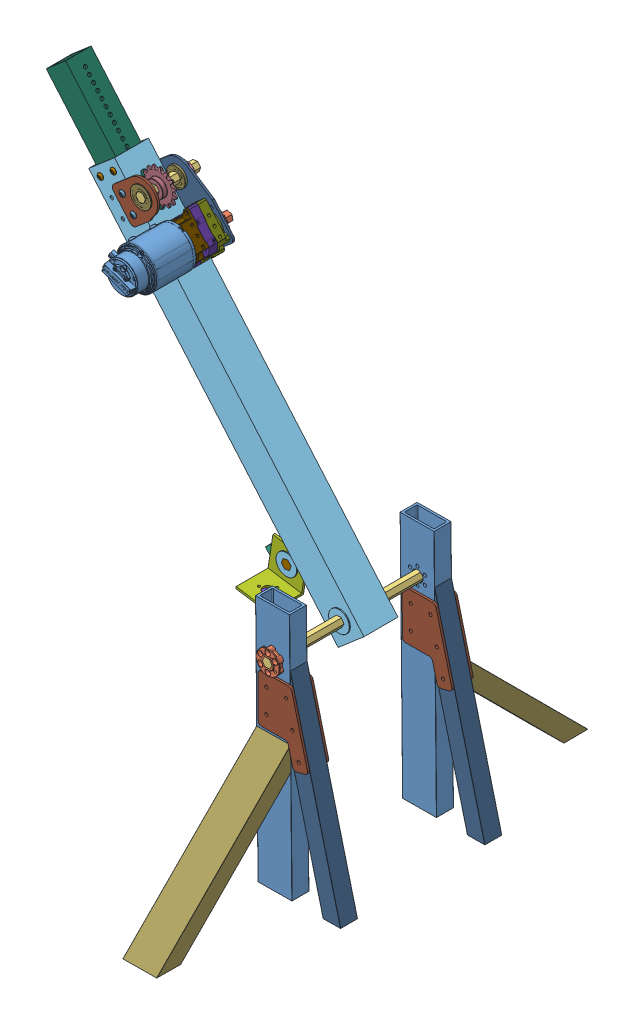
SolidWorks assembly Superstructure, configuration Default. Lengths in mm.
Overall size (550.79 868.94 643.74).
80 component instances, 33 part files, 95 mates.
Components (placement in the parent):
- 3ft 9in Structure Tubing-1: 3ft 9in Structure Tubing [Default] at (63.7822 4129.4809 3.1437) x (0 0 1) z (0.010015 -0.99995 0) size (25.4 50.8 368.3)
- 3ft 9in Structure Tubing-2: 3ft 9in Structure Tubing [Default] at (63.7822 4129.4809 -212.7563) x (0 0 1) z (0.010015 -0.99995 0) size (25.4 50.8 368.3)
- REV Max Hub-3: REV Max Hub [Default] at (39.083 4059.38 -210.5338) x (-0.99995 -0.010015 0) z (0 0 -1) size (34.91 34.92 8.73)
- REV Max Hub-4: REV Max Hub [Default] at (39.083 4059.38 28.5437) x (0.491302 0.870989 0) z (0 0 1) size (34.91 34.92 8.73)
- Dead Axle-1: Dead Axle [Default] at (39.083 4059.38 -219.265) x (0 0 1) z (-0.943614 -0.331047 0) size (256.54 14.38 13.89)
- GOOD Telescoping+Powered+Arm+ASM-3: GOOD Telescoping+Powered+Arm+ASM [Default] at (-316.9253 4473.4855 -96.9323) x (0 0 1) z (-0.65191 0.758296 0) size (167.89 106.2 685.8)
  - Telescoping+Powered+Arm+ASM.stp-1: Telescoping+Powered+Arm+ASM.stp [Default] at origin size (82.02 101.6 1168.4)
    - 2x2tube ASM.stp-1: 2x2tube ASM.stp [Default] at origin size (55.93 50.8 914.4)
      - Slider_Blocks.stp-1: Slider_Blocks.stp [Default] at origin size (17.4 47.5 12.7)
        - Slider_Blocks_4.stp-1: Slider_Blocks_4.stp [Default] at (-0.0635 1254.125 -781.05) x (0 1 0) z (-1 0 0) size (47.5 12.7 17.4)
      - Slider_Blocks_1.stp-1: Slider_Blocks_1.stp [Default] at origin size (17.4 47.5 12.7)
        - Slider_Blocks_4.stp-1: Slider_Blocks_4.stp [Default] at (-0.0635 1254.125 -908.05) x (0 1 0) z (-1 0 0) size (47.5 12.7 17.4)
      - Slider_Blocks_2.stp-1: Slider_Blocks_2.stp [Default] at origin size (17.4 47.5 12.7)
        - Slider_Blocks_4.stp-1: Slider_Blocks_4.stp [Default] at (0.0635 -1254.125 -781.05) x (0 -1 0) z (1 0 0) size (47.5 12.7 17.4)
      - Slider_Blocks_3.stp-1: Slider_Blocks_3.stp [Default] at origin size (17.4 47.5 12.7)
        - Slider_Blocks_4.stp-1: Slider_Blocks_4.stp [Default] at (0.0635 -1254.125 -908.05) x (0 -1 0) z (1 0 0) size (47.5 12.7 17.4)
      - 2x2 long Stick.stp-1: 2x2 long Stick.stp [Default] at origin size (50.8 50.8 914.4)
      - 95185A190_Zinc-Plated Steel Press-Fit Nut for Sheet Metal.stp-1: 95185A190_Zinc-Plated Steel Press-Fit Nut for Sheet Metal.stp [Default] at (-21.5265 12.7 -38.1) x (0 0 -1) z (1 0 0) size (8.64 8.64 3.71)
      - 95185A190_Zinc-Plated Steel Press-Fit Nut for Sheet Metal.stp-2: 95185A190_Zinc-Plated Steel Press-Fit Nut for Sheet Metal.stp [Default] at (-21.5265 12.7 -63.5) x (0 0 -1) z (1 0 0) size (8.64 8.64 3.71)
      - 95185A190_Zinc-Plated Steel Press-Fit Nut for Sheet Metal.stp-3: 95185A190_Zinc-Plated Steel Press-Fit Nut for Sheet Metal.stp [Default] at (-21.5265 12.7 -88.9) x (0 0 -1) z (1 0 0) size (8.64 8.64 3.71)
      - 95185A190_Zinc-Plated Steel Press-Fit Nut for Sheet Metal.stp-4: 95185A190_Zinc-Plated Steel Press-Fit Nut for Sheet Metal.stp [Default] at (-21.5265 12.7 -114.3) x (0 0 -1) z (1 0 0) size (8.64 8.64 3.71)
      - 95185A190_Zinc-Plated Steel Press-Fit Nut for Sheet Metal(Mirror).stp-1: 95185A190_Zinc-Plated Steel Press-Fit Nut for Sheet Metal(Mirror).stp [Default] at (21.5265 12.7 -38.1) x (0 0 -1) z (1 0 0) size (8.64 8.64 3.71)
      - 95185A190_Zinc-Plated Steel Press-Fit Nut for Sheet Metal(Mirror).stp-2: 95185A190_Zinc-Plated Steel Press-Fit Nut for Sheet Metal(Mirror).stp [Default] at (21.5265 12.7 -63.5) x (0 0 -1) z (1 0 0) size (8.64 8.64 3.71)
      - 95185A190_Zinc-Plated Steel Press-Fit Nut for Sheet Metal(Mirror).stp-3: 95185A190_Zinc-Plated Steel Press-Fit Nut for Sheet Metal(Mirror).stp [Default] at (21.5265 12.7 -88.9) x (0 0 -1) z (1 0 0) size (8.64 8.64 3.71)
      - 95185A190_Zinc-Plated Steel Press-Fit Nut for Sheet Metal(Mirror).stp-4: 95185A190_Zinc-Plated Steel Press-Fit Nut for Sheet Metal(Mirror).stp [Default] at (21.5265 12.7 -114.3) x (0 0 -1) z (1 0 0) size (8.64 8.64 3.71)
      - 91255A025_Button Head Hex Drive Screw.stp-1: 91255A025_Button Head Hex Drive Screw.stp [Default] at (-24.3014 -12.7 -12.7) x (0 0 1) z (-1 0 0) size (9.16 9.16 7.33)
      - 91255A025_Button Head Hex Drive Screw.stp-2: 91255A025_Button Head Hex Drive Screw.stp [Default] at (-24.3014 12.7 -12.7) x (0 0 1) z (-1 0 0) size (9.16 9.16 7.33)
      - 91255A025_Button Head Hex Drive Screw.stp-3: 91255A025_Button Head Hex Drive Screw.stp [Default] at (-24.3014 12.7 -139.7) x (0 0 1) z (-1 0 0) size (9.16 9.16 7.33)
      - 91255A025_Button Head Hex Drive Screw.stp-4: 91255A025_Button Head Hex Drive Screw.stp [Default] at (-24.3014 -12.7 -139.7) x (0 0 1) z (-1 0 0) size (9.16 9.16 7.33)
      - 91255A025_Button Head Hex Drive Screw(Mirror).stp-1: 91255A025_Button Head Hex Drive Screw(Mirror).stp [Default] at (24.3014 -12.7 -12.7) x (0 0 1) z (-1 0 0) size (9.16 9.16 7.33)
      - 91255A025_Button Head Hex Drive Screw(Mirror).stp-2: 91255A025_Button Head Hex Drive Screw(Mirror).stp [Default] at (24.3014 12.7 -12.7) x (0 0 1) z (-1 0 0) size (9.16 9.16 7.33)
      - 91255A025_Button Head Hex Drive Screw(Mirror).stp-3: 91255A025_Button Head Hex Drive Screw(Mirror).stp [Default] at (24.3014 12.7 -139.7) x (0 0 1) z (-1 0 0) size (9.16 9.16 7.33)
      - 91255A025_Button Head Hex Drive Screw(Mirror).stp-4: 91255A025_Button Head Hex Drive Screw(Mirror).stp [Default] at (24.3014 -12.7 -139.7) x (0 0 1) z (-1 0 0) size (9.16 9.16 7.33)
    - gear box.stp-1: gear box.stp [Default] at (-25.4 12.7 -38.1) x (0 -1 0) z (1 0 0) size (76.2 113.36 82.02)
      - Selft_drive_Guesset.stp-1: Selft_drive_Guesset.stp [Default] at (12.7 -38.1 25.4) x (0 0 1) z (0 -1 0) size (3.18 76.2 111.91)
        - Selft_drive_Guesset_1.stp-1: Selft_drive_Guesset_1.stp [Default] at (0 -1254.125 -508) x (0 -1 0) z (1 0 0) size (76.2 111.91 3.18)
      - Selfie_drive_guesset_small.stp-1: Selfie_drive_guesset_small.stp [Default] at (12.7 -38.1 25.4) x (0 0 1) z (0 -1 0) size (3.18 64.58 50.8)
        - Selfie_drive_guesset_small_1.stp-1: Selfie_drive_guesset_small_1.stp [Default] at (50.8 -1254.125 -508) x (0 -1 0) z (1 0 0) size (64.58 50.8 3.17)
      - Ball Bearing.stp-1: Ball Bearing.stp [Default] at (-28.067 11.1125 -0.7937) x (1 0 0) z (0 0 -1) size (31.12 31.12 7.94)
      - Ball Bearing.stp-2: Ball Bearing.stp [Default] at (-28.067 11.1125 51.5938) size (31.12 31.12 7.94)
      - hex shaft.stp-1: hex shaft.stp [Default] at (-28.067 11.1125 -388.9375) size (13.74 12.75 73.03) (hidden)
      - 93286A013_Aluminum Washer.stp-1: 93286A013_Aluminum Washer.stp [Default] at (-28.067 11.1125 -5.334) x (0 0 1) z (-1 0 0) size (1.14 17.48 17.48) (hidden)
      - 93286A013_Aluminum Washer.stp-2: 93286A013_Aluminum Washer.stp [Default] at (-28.067 11.1125 68.834) x (0 0 -1) z (1 0 0) size (1.14 17.48 17.48) (hidden)
      - 91255A535_Button Head Hex Drive Screw.stp-1: 91255A535_Button Head Hex Drive Screw.stp [Default] at (-28.067 11.1125 -2.8194) x (1 0 0) z (0 0 -1) size (11.09 11.09 12.88) (hidden)
      - 91255A535_Button Head Hex Drive Screw.stp-2: 91255A535_Button Head Hex Drive Screw.stp [Default] at (-28.067 11.1125 66.3194) size (11.09 11.09 12.88) (hidden)
      - 15 Tooth Sprocket.stp-1: 15 Tooth Sprocket.stp [Default] at (-28.067 11.1125 26.397) size (50.31 50.58 10.68)
      - 91255A262_Button Head Hex Drive Screw.stp-1: 91255A262_Button Head Hex Drive Screw.stp [Default] at (0 76.2 -0.489) x (1 0 0) z (0 0 -1) size (9.16 9.16 10.5)
      - 91255A262_Button Head Hex Drive Screw.stp-2: 91255A262_Button Head Hex Drive Screw.stp [Default] at (0 50.8 -0.489) x (1 0 0) z (0 0 -1) size (9.16 9.16 10.5)
      - 91255A262_Button Head Hex Drive Screw.stp-3: 91255A262_Button Head Hex Drive Screw.stp [Default] at (0 25.4 51.2889) size (9.16 9.16 10.5)
      - 91255A262_Button Head Hex Drive Screw.stp-4: 91255A262_Button Head Hex Drive Screw.stp [Default] at (0 0 -0.489) x (1 0 0) z (0 0 -1) size (9.16 9.16 10.5)
      - 91255A262_Button Head Hex Drive Screw.stp-5: 91255A262_Button Head Hex Drive Screw.stp [Default] at (0 25.4 -0.489) x (1 0 0) z (0 0 -1) size (9.16 9.16 10.5)
      - 91255A262_Button Head Hex Drive Screw.stp-6: 91255A262_Button Head Hex Drive Screw.stp [Default] at (0 0 51.2889) size (9.16 9.16 10.5)
    - 1.5 slide tube.stp-1: 1.5 slide tube.stp [Default] at (-19.05 -19.05 -914.4) size (38.1 38.1 1168.4)
  - gearbox 1-1: gearbox 1 [Default] at (-15.875 50.8 -111.9149) x (-1 0 0) z (0 0 -1) size (23.2 50.8 61.92)
  - gearbox 2-2: gearbox 2 [Default] at (0 50.8 -111.9149) x (0 0 1) z (-1 0 0) size (61.91 50.8 16.85)
  - gearbox 3-1: gearbox 3 [Default] at (15.875 50.8 -111.9149) x (0 0 1) z (-1 0 0) size (61.91 50.8 19.05)
  - Falcon 500, Powered by Talon FX (Rev 3) (217-6515).step-1: Falcon 500, Powered by Talon FX (Rev 3) (217-6515).step [Default] at (86.15 50.8 -111.9149) x (0 0 1) z (-1 0 0) size (62.05 60 125.3)
  - 1in hex axle-1: 1in hex axle [Default] at (-52.3875 50.8003 -111.9276) x (0 -0.481071 -0.876682) z (1 0 0) size (14.66 12.7 38.1)
  - 3.25in hex axle-1: 3.25in hex axle [Default] at (-52.3875 40.7543 -49.2345) x (0 -0.866025 0.5) z (1 0 0) size (14.66 12.7 82.55)
  - 18 tooth sprocket.step-1: 18 tooth sprocket.step [Default] at (-34.29 50.8025 -112.0292) x (0 -0.481071 -0.876682) z (1 0 0) size (39.38 39.82 10.29)
  - 18 tooth sprocket.step-2: 18 tooth sprocket.step [Default] at (-31.5595 40.8051 -49.1465) x (0 0 1) z (-1 0 0) size (39.38 39.82 10.29)
  - Hex Bearing-1: Hex Bearing [Default] at (-18.9967 0 -546.1) x (0 0.175573 0.984466) z (-1 0 0) size (31.12 31.12 7.93)
  - Hex Bearing-2: Hex Bearing [Default] at (18.9967 0 -546.1) x (0 0.878416 0.477897) z (1 0 0) size (31.12 31.12 7.93)
- Arm Mounting Place-3: Arm Mounting Place [Default] at (-51.8162 4048.2259 -109.6323) x (0 0 1) z (-0.65191 0.758296 0) size (127 87.71 84.27)
  - 2x2x2 with holes-1: 2x2x2 with holes [Default] at origin size (25.4 50.8 50.8)
  - Hinge L Bracket-1: Hinge L Bracket [Default] at (-50.8 21.4015 -11.4442) x (1 0 0) z (0 -0.650005 0.75993) size (50.8 50.8 50.8)
  - Hinge L Bracket-2: Hinge L Bracket [Default] at (76.2 -11.6187 27.1602) x (-1 0 0) z (0 0.650005 -0.75993) size (50.8 50.8 50.8)
  - Hex Bearing-1: Hex Bearing [Default] at (3.2283 25.4 25.4) x (0 0 1) z (-1 0 0) size (31.12 31.12 7.93)
  - Hex Bearing-2: Hex Bearing [Default] at (22.1717 25.4 25.4) x (0 0 -1) z (1 0 0) size (31.12 31.12 7.93)
  - 6350K151_3 8 -12 Thread Flange Nut for Fast-Travel Ultra-Precision Lead Screw-1: 6350K151_3 8 -12 Thread Flange Nut for Fast-Travel Ultra-Precision Lead Screw [6350K151] at (-27.9908 4.8914 7.858) x (0 -0.75993 -0.650005) z (-0.733019 0.442138 -0.51691) size (26.34 28.18 28.18)
  - 6350K151_3 8 -12 Thread Flange Nut for Fast-Travel Ultra-Precision Lead Screw-2: 6350K151_3 8 -12 Thread Flange Nut for Fast-Travel Ultra-Precision Lead Screw [6350K151] at (53.3908 4.8914 7.858) x (0 -0.75993 -0.650005) z (0.222567 0.633701 -0.740869) size (26.34 28.18 28.18)
  - 2.5in Axle-1: 2.5in Axle [Default] at (30.099 25.4 25.4) x (0 0.979457 0.201651) z (0 -0.201651 0.979457) size (13.92 34.29 14.36)
- Back Support-1: Back Support [Default] at (-97.4015 4590.0884 -187.3563) x (0 0 -1) z (0.246763 -0.969076 0) size (25.4 25.4 304.68)
- Back Support-2: Back Support [Default] at (-97.0045 4590.0924 28.5437) x (0 0 -1) z (0.246763 -0.969076 0) size (25.4 25.4 304.68)
- Back Support Bracket-1: Back Support Bracket [Default] at (22.9442 3912.6818 28.5437) x (0.999975 0.007087 0) z (0 0 1) size (73.62 105.21 3.17)
- Back Support Bracket-2: Back Support Bracket [Default] at (22.9442 3912.6818 -0.0313) x (0.999975 0.007087 0) z (0 0 1) size (73.62 105.21 3.17)
- Back Support Bracket-3: Back Support Bracket [Default] at (22.5704 3912.5866 -187.3563) x (0.999975 0.007087 0) z (0 0 1) size (73.62 105.21 3.17)
- Back Support Bracket-4: Back Support Bracket [Default] at (22.5704 3912.5866 -215.9313) x (0.999975 0.007087 0) z (0 0 1) size (73.62 105.21 3.17)
- Angled 18in 2x1-1: Angled 18in 2x1 [Default] at (16.6605 3761.9454 -413.3497) x (0.007081 -0.707071 0.707107) z (-0.007081 0.707071 0.707107) size (25.4 50.8 283.68)
- Angled 18in 2x1-2: Angled 18in 2x1 [Default] at (14.6641 3961.2865 28.5437) x (0.007125 -0.711481 -0.70267) z (0.007037 -0.702634 0.711516) size (25.4 50.8 283.68)
Mates (geometry in assembly coordinates):
- Coincident11: coincident: plane of 3ft 9in Structure Tubing-1 through (82.0968 2300.7726 3.3977) normal (0.99995 0.010015 0); plane of 3ft 9in Structure Tubing-2 through (82.0968 2300.7726 -212.5023) normal (0.99995 0.010015 0)
- Coincident15: coincident anti-aligned: plane of 3ft 9in Structure Tubing-1 through (63.5282 4129.4784 3.3977) normal (-0.010015 0.99995 0); plane of Top Connector-1 through (80.3407 4110.2202 1616.0437) normal (0.010015 -0.99995 0)
- Coincident16: coincident aligned: plane of 3ft 9in Structure Tubing-1 through (31.2993 2300.2639 3.3977) normal (-0.99995 -0.010015 0); plane of Top Connector-1 through (29.5433 4109.7115 1616.0437) normal (-0.99995 -0.010015 0)
- Coincident13: coincident aligned: plane of 3ft 9in Structure Tubing-2 through (81.8428 2300.7701 -212.7563) normal (0 0 -1); plane of Back Support-1 through (354.1246 2817.9051 -212.7563) normal (0 0 -1)
- Coincident17: coincident anti-aligned: plane of Back Support-1 through (354.1246 2817.9051 -187.3563) normal (0 0 1); plane of Back Support Connector-1 through (222.6392 3263.2808 -187.3563) normal (0 0 -1)
- Coincident18: coincident aligned: plane of Back Support-1 through (378.493 2824.1102 -187.6103) normal (0.969076 0.246763 0); plane of Back Support Connector-1 through (246.9894 3269.557 1641.4437) normal (0.968351 0.249592 0)
- Distance3: distance = 228.6 mm: line of Back Support Connector-1 through (246.9894 3269.557 3.6517) axis (0 0 -1); line of Back Support-2 through (140.0879 3761.9266 28.2897) axis (0 0 -1)
- Coincident21: coincident anti-aligned: plane of Back Support-2 through (354.5216 2817.909 3.1437) normal (0 0 -1); plane of Back Support Connector-2 through (137.2722 3593.4645 3.1437) normal (0 0 1)
- Coincident22: coincident aligned: plane of Back Support-2 through (378.89 2824.1141 28.2897) normal (0.969076 0.246763 0); plane of Back Support Connector-2 through (161.805 3600.0501 1640.9357) normal (0.968351 0.249592 0)
- Distance4: distance = 228.6 mm: line of Back Support Connector-2 through (155.5921 3624.1543 3.1437) axis (0 0 -1); line of Back Support-2 through (64.9033 4057.1885 28.2897) axis (0 0 -1)
- Coincident29: coincident anti-aligned: plane of 3ft 9in Structure Tubing-2 through (81.8428 2300.7701 -212.7563) normal (0 0 -1); plane of REV Max Hub-1 through (63.7027 4115.5685 -236.4913) normal (0 0 1)
- Coincident32: coincident anti-aligned: plane of 3ft 9in Structure Tubing-1 through (81.8428 2300.7701 28.5437) normal (0 0 1); plane of REV Max Hub-2 through (63.7027 4115.5685 4.8087) normal (0 0 -1)
- Concentric5: concentric anti-aligned: circle of 3ft 9in Structure Tubing-1; circle of REV Max Hub-2
- Concentric6: concentric anti-aligned: circle of 3ft 9in Structure Tubing-1; circle of REV Max Hub-2
- Coincident47: coincident anti-aligned: plane of 3ft 9in Structure Tubing-1 through (81.8428 2300.7701 28.5437) normal (0 0 1); plane of REV Max Hub-4 through (39.083 4059.38 28.5437) normal (0 0 -1)
- Concentric14: concentric: circle of 3ft 9in Structure Tubing-2; circle of REV Max Hub-3
- Concentric15: concentric: circle of 3ft 9in Structure Tubing-2; circle of REV Max Hub-3
- Concentric16: concentric anti-aligned: circle of 3ft 9in Structure Tubing-1; circle of REV Max Hub-4
- Concentric17: concentric anti-aligned: circle of 3ft 9in Structure Tubing-1; circle of REV Max Hub-4
- Coincident54: coincident aligned: plane of 3ft 9in Structure Tubing-1 through (81.8428 2300.7701 28.5437) normal (0 0 1); plane of Top Connector-1 through (54.8148 4122.6652 28.5437) normal (0 0 1)
- Coincident56: coincident aligned: plane of Back Support-2 through (378.89 2824.1141 28.2897) normal (0.969076 0.246763 0); plane of Back Support Bracket-1 through (103.8167 3894.2745 35.9237) normal (0.970802 0.239882 0)
- Parallel2: parallel: plane of Back Support-1 through (139.6909 3761.9227 -115.9823) normal (0.010015 -0.99995 0); plane of Back Support-2 through (140.0879 3761.9266 99.9177) normal (0.010015 -0.99995 0)
- Coincident82: coincident aligned: plane of 3ft 9in Structure Tubing-1 through (81.8428 2300.7701 28.5437) normal (0 0 1); plane of Back Support-4 through (506.9772 2160.1244 28.5437) normal (0 0 1)
- Coincident87: coincident aligned: plane of 3ft 9in Structure Tubing-1 through (31.2993 2300.2639 3.3977) normal (-0.99995 -0.010015 0); plane of Back Support Bracket-1 through (52.8391 3771.8342 35.9237) normal (-1 0.000007 0)
- Distance8: distance = 244.348 mm aligned: plane of Back Support Bracket-1 through (59.19 3899.1016 35.9237) normal (0.000007 1 0); plane of Top Connector-1 through (103.6419 4143.4492 1620.2487) normal (0.000007 1 0)
- Coincident97: coincident anti-aligned: plane of 3ft 9in Structure Tubing-1 through (63.5282 4129.4784 3.3977) normal (-0.010015 0.99995 0); plane of Top Connector-1 through (80.3407 4110.2202 1616.0437) normal (0.010015 -0.99995 0)
- Coincident101: coincident aligned: plane of Back Support Connector-1 through (246.9894 3269.557 1641.4437) normal (0.968351 0.249592 0); plane of Back Support-4 through (531.3274 2166.4007 28.2897) normal (0.968351 0.249592 0)
- Coincident102: coincident aligned: plane of Back Support Connector-2 through (161.805 3600.0501 1640.9357) normal (0.968351 0.249592 0); plane of Back Support-4 through (531.3274 2166.4007 28.2897) normal (0.968351 0.249592 0)
- Coincident104: coincident anti-aligned: plane of 3ft 9in Structure Tubing-2 through (82.0968 2300.7726 -212.5023) normal (0.99995 0.010015 0); plane of Back Support-5 through (92.1824 3768.4012 -115.9823) normal (-0.99995 -0.010015 0)
- Coincident105: coincident aligned: plane of 3ft 9in Structure Tubing-2 through (81.8428 2300.7701 -212.7563) normal (0 0 -1); plane of Back Support-5 through (506.9772 2160.1244 -212.7563) normal (0 0 -1)
- Coincident106: coincident aligned: line of Back Support-4 through (91.122 3874.2813 28.2897) axis (0 0 -1); line of Back Support-5 through (91.122 3874.2813 -187.6103) axis (0 0 -1)
- Coincident107: coincident: plane of 3ft 9in Structure Tubing-2 through (113.6584 3058.8018 -206.8417) normal (0.010015 -0.99995 0); plane of Angled 18in 2x1-1 through (113.6584 3058.8018 -413.6076) normal (0.010015 -0.99995 0)
- Coincident108: coincident anti-aligned: plane of 3ft 9in Structure Tubing-1 through (31.2993 2300.2639 3.3977) normal (-0.99995 -0.010015 0); plane of Side Bracket-1 through (45.7858 3328.4633 48.5425) normal (0.99995 0.010015 0)
- Coincident109: coincident aligned: plane of 3ft 9in Structure Tubing-1 through (81.8428 2300.7701 3.1437) normal (0 0 -1); plane of Side Bracket-1 through (42.6867 3320.8764 3.1437) normal (0 0 -1)
- Coincident115: coincident anti-aligned: plane of 3ft 9in Structure Tubing-1 through (82.0968 2300.7726 3.3977) normal (0.99995 0.010015 0); plane of Side Bracket-2 through (96.6078 3326.5282 50.0172) normal (-0.99995 -0.010015 0)
- Coincident121: coincident anti-aligned: plane of 3ft 9in Structure Tubing-2 through (31.2993 2300.2639 -212.5023) normal (-0.99995 -0.010015 0); plane of Side Bracket-3 through (45.7867 3328.3782 -226.759) normal (0.99995 0.010015 0)
- Coincident124: coincident anti-aligned: plane of REV Max Hub-3 through (35.3534 4065.693 -210.5338) normal (0.010015 -0.99995 0); plane of Dead Axle-1 through (42.6854 4065.7664 37.275) normal (-0.010015 0.99995 0)
- Coincident125: coincident anti-aligned: plane of REV Max Hub-3 through (42.6854 4065.7664 -210.5338) normal (-0.860975 -0.508648 0); plane of Dead Axle-1 through (46.415 4059.4535 37.275) normal (0.860975 0.508648 0)
- Coincident126: coincident aligned: plane of REV Max Hub-3 through (39.083 4059.38 -219.265) normal (0 0 -1); plane of Dead Axle-1 through (39.083 4059.38 -219.265) normal (0 0 -1)
- Coincident135: coincident anti-aligned: plane of Dead Axle-1 through (35.3534 4065.693 37.275) normal (-0.870989 0.491302 0); plane of GOOD Telescoping+Powered+Arm+ASM-2/am-2986 FR8ZZ Hex Bearing.step-1 through (66.8965 4047.2081 -98.3565) normal (0.866022 -0.500006 0)
- Coincident136: coincident anti-aligned: plane of Dead Axle-1 through (35.4806 4052.9936 37.275) normal (0.010015 -0.99995 0); plane of GOOD Telescoping+Powered+Arm+ASM-2/am-2986 FR8ZZ Hex Bearing.step-1 through (77.8949 4040.858 -98.3565) normal (0.000007 1 0)
- Coincident137: coincident anti-aligned: plane of Back Support Connector-2 through (137.2722 3593.4645 3.1437) normal (0 0 1); plane of Back Support-4 through (506.9772 2160.1244 3.1437) normal (0 0 -1)
- Coincident138: coincident anti-aligned: plane of Back Support Connector-1 through (222.6392 3263.2808 -187.3563) normal (0 0 -1); plane of Back Support-5 through (506.9772 2160.1244 -187.3563) normal (0 0 1)
- Coincident139: coincident: plane of Dead Axle-1 through (42.6854 4065.7664 37.275) normal (-0.010015 0.99995 0); plane of GOOD Telescoping+Powered+Arm+ASM-2/Hex Bearing-2 through (11.1788 4068.0671 -60.044) normal (0.010015 -0.99995 0)
- Coincident140: coincident: plane of Dead Axle-1 through (35.3534 4065.693 37.275) normal (-0.870989 0.491302 0); plane of GOOD Telescoping+Powered+Arm+ASM-2/Hex Bearing-2 through (7.5764 4061.6807 -60.044) normal (0.870989 -0.491302 0)
- Distance9: distance = 63.1877 mm: plane of GOOD Telescoping+Powered+Arm+ASM-2/Hex Bearing-2 through (-0.6483 4061.5983 -60.044) normal (0 0 1); plane of 3ft 9in Structure Tubing-1 through (81.8428 2300.7701 3.1437) normal (0 0 -1)
- Coincident142: coincident anti-aligned: plane of Back Support-4 through (506.9772 2160.1244 28.5437) normal (0 0 1); plane of REV Max Hub-5 through (145.89 3669.28 5.4712) normal (0 0 -1)
- Concentric18: concentric aligned: circle of Back Support-4; circle of REV Max Hub-5
- Concentric19: concentric anti-aligned: circle of Back Support-4; circle of Axle Holder-1
- Coincident145: coincident anti-aligned: plane of Back Support-4 through (506.9772 2160.1244 28.5437) normal (0 0 1); plane of Axle Holder-1 through (135.6248 3649.7215 28.5437) normal (0 0 -1)
- Coincident147: coincident anti-aligned: plane of Axle Holder-1 through (140.3693 3653.9419 3.1437) normal (-0.747162 -0.664642 0); plane of 10in Axle-1 through (142.806 3651.2027 38.7037) normal (0.747162 0.664642 0)
- Coincident148: coincident anti-aligned: plane of Axle Holder-1 through (134.342 3655.9405 3.1437) normal (0.202016 -0.979382 0); plane of 10in Axle-1 through (137.9326 3656.6812 38.7037) normal (-0.202016 0.979382 0)
- Coincident155: coincident aligned: plane of 3ft 9in Structure Tubing-2 through (81.8428 2300.7701 -212.7563) normal (0 0 -1); plane of Top Connector-1 through (54.8148 4122.6652 -212.7563) normal (0 0 -1)
- Coincident182: coincident anti-aligned: plane of 10in Axle-1 through (130.7514 3655.1999 38.7037) normal (-0.949178 0.31474 0); plane of Motor Housing Assembly-3/Hex Bearing-4 through (139.7422 3665.2839 3.433) normal (0.998608 0.052752 0)
- Coincident183: coincident anti-aligned: plane of 10in Axle-1 through (137.9326 3656.6812 38.7037) normal (-0.202016 0.979382 0); plane of Motor Housing Assembly-3/Hex Bearing-4 through (139.3554 3672.6061 3.433) normal (0.544988 -0.838444 0)
- Distance13: distance = 13.3563 mm anti-aligned: plane of Motor Housing Assembly-3/Hex Bearing-3 through (159.7548 3662.2228 -169.795) normal (0 0 -1); plane of Back Support-5 through (506.9772 2160.1244 -187.3563) normal (0 0 1)
- Coincident184: coincident anti-aligned: plane of GOOD Telescoping+Powered+Arm+ASM-2/Telescoping+Powered+Arm+ASM.stp-1/2x2tube ASM.stp-1/2x2 long Stick.stp-1 through (-156.2704 3685.3161 -61.568) normal (0.883158 -0.469076 0); plane of 2x2x2 with holes-1 through (-72.4243 3718.1193 -108.163) normal (-0.878412 0.477903 0)
- Coincident185: coincident aligned: plane of GOOD Telescoping+Powered+Arm+ASM-2/Telescoping+Powered+Arm+ASM.stp-1/2x2tube ASM.stp-1/2x2 long Stick.stp-1 through (-201.1348 3709.1452 -61.568) normal (0 0 1); plane of 2x2x2 with holes-1 through (-27.8009 3693.8418 -57.363) normal (0 0 1)
- Distance14: distance = 50.8 mm aligned: plane of 2x2x2 with holes-1 through (-27.8009 3693.8418 -108.163) normal (-0.477903 -0.878412 0); plane of GOOD Telescoping+Powered+Arm+ASM-2/Telescoping+Powered+Arm+ASM.stp-1/2x2tube ASM.stp-1/2x2 long Stick.stp-1 through (-178.7026 3697.2307 -86.968) normal (-0.469076 -0.883158 0)
- Coincident196: coincident anti-aligned: plane of 10in Axle-1 through (140.4982 3644.243 38.7037) normal (0.949178 -0.31474 0); plane of Motor Housing Assembly-4/Hex Bearing-3 through (142.806 3651.2027 -0.3377) normal (-0.949178 0.31474 0)
- Coincident199: coincident anti-aligned: plane of 10in Axle-1 through (137.9326 3656.6812 38.7037) normal (-0.202016 0.979382 0); plane of Motor Housing Assembly-4/Hex Bearing-3 through (130.7514 3655.1999 -0.3377) normal (0.202016 -0.979382 0)
- Coincident201: coincident anti-aligned: plane of Angled 18in 2x1-1 through (3.712 5054.8578 879.9868) normal (-0.99995 -0.010015 0); plane of Side Bracket-3 through (45.7867 3328.3782 -226.759) normal (0.99995 0.010015 0)
- Coincident206: coincident aligned: plane of Angled 18in 2x1-1 through (3.9642 5055.0399 879.8072) normal (-0.007081 0.707071 -0.707107); plane of Side Bracket-3 through (45.1207 3394.8783 -208.5097) normal (-0.005215 0.520697 -0.853726)
- Coincident207: coincident aligned: plane of Top Connector-1 through (80.3407 4110.2202 1616.0437) normal (0.010015 -0.99995 0); circle of 3ft 9in Structure Tubing-2
- Coincident208: coincident: plane of REV Max Hub-4 through (39.083 4059.38 37.275) normal (0 0 1); plane of Dead Axle-1 through (39.083 4059.38 37.275) normal (0 0 1)
- Coincident216: coincident: plane of Dead Axle-1 through (42.6854 4065.7664 37.275) normal (-0.010015 0.99995 0); plane of GOOD Telescoping+Powered+Arm+ASM-3/Hex Bearing-1 through (42.6854 4065.7664 -123.8563) normal (0.010015 -0.99995 0)
- Coincident217: coincident: plane of Dead Axle-1 through (35.3534 4065.693 37.275) normal (-0.870989 0.491302 0); plane of GOOD Telescoping+Powered+Arm+ASM-3/Hex Bearing-1 through (35.3534 4065.693 -123.8563) normal (0.870989 -0.491302 0)
- Distance20: distance = 63.5 mm: plane of GOOD Telescoping+Powered+Arm+ASM-3/Hex Bearing-1 through (31.1697 4072.7747 -123.8563) normal (0 0 -1); plane of 3ft 9in Structure Tubing-2 through (81.8428 2300.7701 -187.3563) normal (0 0 1)
- Coincident219: coincident anti-aligned: plane of 3ft 9in Structure Tubing-2 through (81.8428 2300.7701 -212.7563) normal (0 0 -1); plane of Angled 18in 2x1-3 through (81.0087 4043.528 -212.7563) normal (0 0 1)
- Coincident220: coincident aligned: plane of 3ft 9in Structure Tubing-2 through (82.0968 2300.7726 -212.5023) normal (0.99995 0.010015 0); plane of Angled 18in 2x1-3 through (68.4438 5298.1337 520.1532) normal (0.99995 0.010015 0)
- Distance21: distance = 17.78 mm: line of Angled 18in 2x1-3 through (29.9753 4091.9349 -212.7563) axis (0.99995 0.010015 0); line of 3ft 9in Structure Tubing-2 through (13.2387 4128.9747 -212.7563) axis (0.99995 0.010015 0)
- Coincident225: coincident: plane of GOOD Telescoping+Powered+Arm+ASM-3/Telescoping+Powered+Arm+ASM.stp-1/2x2tube ASM.stp-1/2x2 long Stick.stp-1 through (-336.186 4456.9269 -71.5323) normal (-0.758296 -0.65191 0); plane of Arm Mounting Place-3/2x2x2 with holes-1 through (-46.4118 4119.8644 -109.6323) normal (0.758296 0.65191 0)
- Distance22: distance = 38.1 mm: plane of Arm Mounting Place-3/2x2x2 with holes-1 through (-84.9333 4086.7473 -109.6323) normal (0 0 -1); plane of GOOD Telescoping+Powered+Arm+ASM-3/Telescoping+Powered+Arm+ASM.stp-1/2x2tube ASM.stp-1/2x2 long Stick.stp-1 through (-297.6646 4490.044 -71.5323) normal (0 0 1)
- Distance23: distance = 76.2 mm: plane of Arm Mounting Place-3/2x2x2 with holes-1 through (-51.8162 4048.2259 -109.6323) normal (0.65191 -0.758296 0); plane of GOOD Telescoping+Powered+Arm+ASM-3/Telescoping+Powered+Arm+ASM.stp-1/2x2tube ASM.stp-1/2x2 long Stick.stp-1 through (55.6415 4040.1193 -96.9323) normal (0.65191 -0.758296 0)
- Coincident226: coincident: plane of REV Max Hub-4 through (35.4806 4052.9936 28.5437) normal (-0.010015 0.99995 0); plane of Dead Axle-1 through (35.4806 4052.9936 37.275) normal (0.010015 -0.99995 0)
- Coincident227: coincident: plane of 3ft 9in Structure Tubing-2 through (82.0968 2300.7726 -212.5023) normal (0.99995 0.010015 0); line of Back Support-1 through (64.5063 4057.1845 -187.6103) axis (0 0 -1)
- Coincident228: coincident aligned: plane of 3ft 9in Structure Tubing-2 through (81.8428 2300.7701 -212.7563) normal (0 0 -1); plane of Back Support-1 through (354.1246 2817.9051 -212.7563) normal (0 0 -1)
- Coincident230: coincident aligned: plane of 3ft 9in Structure Tubing-2 through (67.4706 3761.1994 -212.7563) normal (0.010015 -0.99995 0); plane of Back Support-1 through (139.6909 3761.9227 -115.9823) normal (0.010015 -0.99995 0)
- Coincident233: coincident aligned: plane of 3ft 9in Structure Tubing-1 through (81.8428 2300.7701 3.1437) normal (0 0 -1); plane of Back Support-2 through (354.5216 2817.909 3.1437) normal (0 0 -1)
- Coincident234: coincident: plane of 3ft 9in Structure Tubing-1 through (67.4706 3761.1994 3.1437) normal (0.010015 -0.99995 0); plane of Back Support-2 through (140.0879 3761.9266 99.9177) normal (0.010015 -0.99995 0)
- Coincident235: coincident anti-aligned: plane of Back Support-2 through (354.5216 2817.909 28.5437) normal (0 0 1); plane of Back Support Bracket-1 through (60.1439 3962.6532 28.5437) normal (0 0 -1)
- Coincident236: coincident aligned: plane of Back Support-2 through (378.89 2824.1141 28.2897) normal (0.969076 0.246763 0); plane of Back Support Bracket-1 through (70.5905 4034.8539 31.7187) normal (0.969076 0.246763 0)
- Coincident237: coincident anti-aligned: plane of Back Support-2 through (354.5216 2817.909 3.1437) normal (0 0 -1); plane of Back Support Bracket-2 through (60.1439 3962.6532 3.1437) normal (0 0 1)
- Coincident238: coincident aligned: plane of Back Support-2 through (378.89 2824.1141 28.2897) normal (0.969076 0.246763 0); plane of Back Support Bracket-2 through (70.5905 4034.8539 3.1437) normal (0.969076 0.246763 0)
- Coincident240: coincident: plane of Back Support-1 through (354.1246 2817.9051 -212.7563) normal (0 0 -1); plane of Back Support Bracket-4 through (59.7701 3962.558 -212.7563) normal (0 0 1)
- Coincident241: coincident aligned: plane of Back Support-1 through (378.493 2824.1102 -187.6103) normal (0.969076 0.246763 0); plane of Back Support Bracket-4 through (70.2167 4034.7587 -212.7563) normal (0.969076 0.246763 0)
- Coincident243: coincident: plane of Back Support-1 through (354.1246 2817.9051 -187.3563) normal (0 0 1); plane of Back Support Bracket-3 through (59.7701 3962.558 -187.3563) normal (0 0 -1)
- Coincident244: coincident aligned: plane of Back Support-1 through (378.493 2824.1102 -187.6103) normal (0.969076 0.246763 0); plane of Back Support Bracket-3 through (70.2167 4034.7587 -184.1813) normal (0.969076 0.246763 0)
- Coincident246: coincident: plane of 3ft 9in Structure Tubing-2 through (81.8428 2300.7701 -212.7563) normal (0 0 -1); plane of Angled 18in 2x1-1 through (67.458 3762.4541 -212.7563) normal (0 0 1)
- Coincident247: coincident: plane of 3ft 9in Structure Tubing-2 through (82.0968 2300.7726 -212.5023) normal (0.99995 0.010015 0); plane of Angled 18in 2x1-1 through (54.5094 5055.3665 879.9868) normal (0.99995 0.010015 0)
- Coincident250: coincident: plane of 3ft 9in Structure Tubing-2 through (67.4706 3761.1994 -212.7563) normal (0.010015 -0.99995 0); plane of Angled 18in 2x1-1 through (67.458 3762.4541 -413.3497) normal (0.010014 -0.99993 -0.006255)
- Coincident251: coincident: plane of 3ft 9in Structure Tubing-2 through (81.8428 2300.7701 -212.7563) normal (0 0 -1); plane of Angled 18in 2x1-1 through (67.458 3762.4541 -212.7563) normal (0 0 1)
- Coincident252: coincident: plane of 3ft 9in Structure Tubing-1 through (81.8428 2300.7701 28.5437) normal (0 0 1); plane of Angled 18in 2x1-2 through (65.4616 3961.7953 28.5437) normal (0 0 -1)
- Coincident254: coincident: plane of 3ft 9in Structure Tubing-1 through (67.4706 3761.1994 3.1437) normal (0.010015 -0.99995 0); plane of Angled 18in 2x1-2 through (67.4704 3761.2159 29.7985) normal (0.010014 -0.99993 0.006255)
- Coincident255: coincident: plane of 3ft 9in Structure Tubing-1 through (31.2993 2300.2639 3.3977) normal (-0.99995 -0.010015 0); plane of Angled 18in 2x1-2 through (27.535 2676.1279 1329.586) normal (-0.99995 -0.010015 0)
